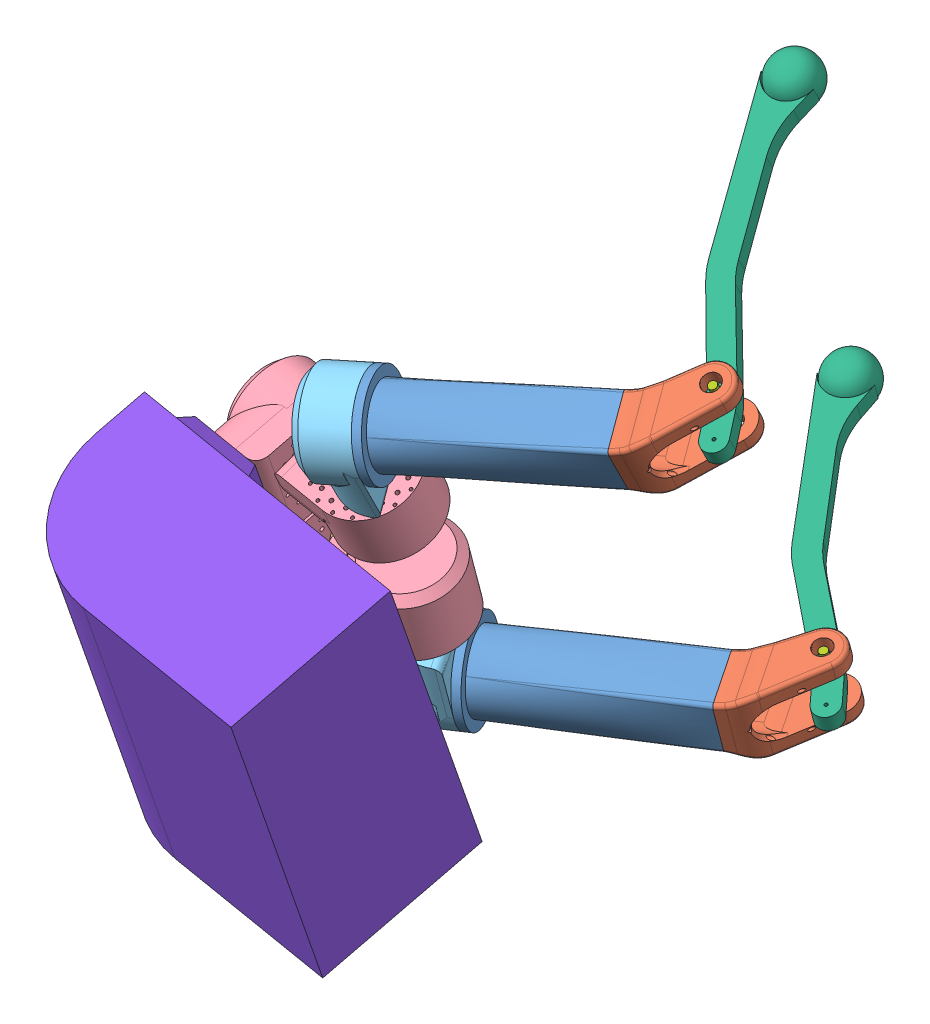
SolidWorks assembly Leg, configuration Default. Lengths in mm.
Overall size (609.04 770.66 944.9).
21 component instances, 8 part files, 41 mates.
Components (placement in the parent):
- Leg_upper-1: Leg_upper [Default] at (371.0813 -601.602 100.7104) x (0.457544 -0.307811 0.83421) z (0.078489 0.94849 0.306929) size (122.65 362.34 115)
  - leg_upper_infront_1-1: leg_upper_infront_1 [Default] at (70.6458 26.5557 199.3325) size (115 250.01 115)
  - leg_upper_infront_2_kfe-1: leg_upper_infront_2_kfe [Default] at (70.6458 26.5557 199.3325) x (0 0 -1) z (1 0 0) size (90 112.35 100.44)
- Output_2-1: Output_2 [Default] at (419.1284 -358.457 248.7598) x (0.995827 -0.088977 0.020306) z (0.04657 0.304055 -0.951516) size (60 8 60)
- Output_2-2: Output_2 [Default] at (343.8426 -295.313 260.2175) x (0.078494 0.948503 0.306888) z (0.105751 0.298179 -0.948634) size (60 8 60)
- Cover_new-1: Cover_new [Default] at (329.9645 -293.8162 259.1409) x (0.071259 0.926481 0.369533) z (0.110755 0.360835 -0.92603) size (115 87.5 130)
- Cover_new-2: Cover_new [Default] at (420.2272 -345.1781 253.0568) x (-0.105755 -0.29822 0.94862) z (0.99129 -0.106915 0.0769) size (115 87.5 130)
- cover-1: cover [Default] at (442.5711 -432.292 208.6587) x (-0.457544 0.307811 -0.83421) z (0.078489 0.94849 0.306929) size (115 63.6 130)
- Leg_Lower_in-1: Leg_Lower_in [Default] at (722.9885 -394.6471 20.617) x (0.638588 -0.284257 0.715125) z (0.765536 0.139872 -0.628005) size (435 60 72.6)
- m10-1: m10 [Default] at (722.9885 -394.6471 20.617) x (0.978231 -0.132605 0.159627) z (0.192105 0.287719 -0.93825) size (10 80 10)
- Leg_upper-2: Leg_upper [Default] at (402.8677 -215.3009 223.9043) x (0.45192 -0.442305 0.774684) z (0.058672 0.88128 0.468939) size (122.65 362.34 115)
  - leg_upper_infront_1-1: leg_upper_infront_1 [Default] at (70.6458 26.5557 199.3325) size (115 250.01 115)
  - leg_upper_infront_2_kfe-1: leg_upper_infront_2_kfe [Default] at (70.6458 26.5557 199.3325) x (0 0 -1) z (1 0 0) size (90 112.35 100.44)
- Output_2-3: Output_2 [Default] at (435.4948 -142.9958 337.3459) x (0.99683 -0.077005 0.019996) z (-0.053733 -0.466279 0.883004) size (60 8 60)
- Output_2-4: Output_2 [Default] at (352.3224 -185.0618 304.192) x (-0.058677 -0.8813 -0.468901) z (-0.117905 -0.460304 0.879897) size (60 8 60)
- Cover_new-3: Cover_new [Default] at (338.4443 -183.565 303.1154) x (0.071259 0.926481 0.369533) z (0.110755 0.360835 -0.92603) size (115 87.5 130)
- Cover_new-4: Cover_new [Default] at (434.6734 -155.3337 330.7808) x (0.117907 0.460343 -0.879876) z (0.99129 -0.106915 0.0769) size (115 87.5 130)
- cover-2: cover [Default] at (470.1271 -66.4594 360.8418) x (0.45192 -0.442305 0.774684) z (-0.058672 -0.88128 -0.468939) size (115 63.6 130)
- Leg_Lower_in-2: Leg_Lower_in [Default] at (752.2584 7.4566 186.6317) x (0.495215 -0.433568 0.752848) z (0.866787 0.188055 -0.461861) size (435 60 72.6)
- m10-2: m10 [Default] at (752.2584 7.4566 186.6317) x (0.982378 -0.134474 0.129807) z (-0.177457 -0.453059 0.87364) size (10 80 10)
- main-2: main [Default] at (417.3182 -308.2316 439.4518) x (0.99129 -0.106915 0.0769) z (0.071259 0.926481 0.369533) size (350 240 400)
Mates (geometry in assembly coordinates):
- Coincident1: coincident anti-aligned: plane of Output_2-2 through (343.8426 -295.313 260.2175) normal (-0.99129 0.106915 -0.0769); plane of Cover_new-1 through (343.8426 -295.313 260.2175) normal (0.99129 -0.106915 0.0769)
- Concentric1: concentric aligned: cylinder of Output_2-2 through (351.7729 -296.1684 260.8327) axis (-0.99129 0.106915 -0.0769) radius 30; cylinder of Cover_new-1 through (343.8426 -295.313 260.2175) axis (-0.99129 0.106915 -0.0769) radius 57.5
- Coincident2: coincident anti-aligned: plane of Output_2-2 through (351.7729 -296.1684 260.8327) normal (0.99129 -0.106915 0.0769); plane of Cover_new-2 through (342.2778 -354.5744 302.0273) normal (-0.99129 0.106915 -0.0769)
- Coincident3: coincident anti-aligned: plane of Output_2-1 through (419.1284 -358.457 248.7598) normal (0.078489 0.94849 0.306929); plane of Cover_new-2 through (419.1284 -358.457 248.7598) normal (-0.078489 -0.94849 -0.306929)
- Concentric2: concentric aligned: cylinder of Output_2-1 through (418.5005 -366.0449 246.3044) axis (0.078489 0.94849 0.306929) radius 30; cylinder of Cover_new-2 through (419.1284 -358.457 248.7598) axis (0.078489 0.94849 0.306929) radius 57.5
- Concentric5: concentric aligned: cylinder of Output_2-2 through (349.3406 -303.0265 282.6513) axis (-0.99129 0.106915 -0.0769) radius 2.1; cylinder of Cover_new-2 through (416.2527 -310.2433 287.842) axis (-0.99129 0.106915 -0.0769) radius 2.25
- Coincident4: coincident anti-aligned: line of Output_2-2 through (352.1202 -280.7044 277.8557) axis (-0.99129 0.106915 -0.0769); line of Cover_new-2 through (362.0331 -281.7735 278.6247) axis (0.99129 -0.106915 0.0769)
- Concentric8: concentric anti-aligned: cylinder of Leg_upper-1/leg_upper_infront_1-1 through (454.6807 -434.343 211.9002) axis (-0.960314 -0.010724 0.278716) radius 57.5; cylinder of cover-1 through (430.6728 -434.6111 218.8681) axis (0.960314 0.010724 -0.278716) radius 57.5
- Coincident5: coincident anti-aligned: plane of Leg_upper-1/leg_upper_infront_1-1 through (445.0775 -434.4502 214.6874) normal (-0.960314 -0.010724 0.278716); plane of cover-1 through (445.0775 -434.4502 214.6874) normal (0.960314 0.010724 -0.278716)
- Coincident6: coincident anti-aligned: plane of Output_2-1 through (418.5005 -366.0449 246.3044) normal (-0.078489 -0.94849 -0.306929); plane of cover-1 through (435.3781 -347.4788 184.6144) normal (0.078489 0.94849 0.306929)
- Concentric9: concentric aligned: line of Output_2-1 through (396.4142 -366.2917 252.7151) axis (0.078489 0.94849 0.306929); cylinder of cover-1 through (390.4805 -437.9976 229.5112) axis (0.078489 0.94849 0.306929) radius 2
- Coincident7: coincident aligned: line of Output_2-1 through (412.7891 -372.4751 267.6359) axis (0.078489 0.94849 0.306929); line of cover-1 through (412.0042 -381.96 264.5666) axis (0.078489 0.94849 0.306929)
- Concentric10: concentric aligned: cylinder of Leg_upper-1/leg_upper_infront_2_kfe-1 through (761.8161 -375.4378 97.94) axis (-0.078489 -0.94849 -0.306929) radius 11; circle of Leg_Lower_in-1
- Coincident9: coincident anti-aligned: plane of cover-1 through (445.0775 -434.4502 214.6874) normal (0.078489 0.94849 0.306929); plane of Leg_Lower_in-1 through (758.2841 -418.1199 84.1282) normal (-0.078489 -0.94849 -0.306929)
- Coincident12: coincident aligned: plane of Leg_upper-1/leg_upper_infront_1-1 through (445.0775 -434.4502 214.6874) normal (0.078489 0.94849 0.306929); plane of cover-1 through (445.0775 -434.4502 214.6874) normal (0.078489 0.94849 0.306929)
- Concentric11: concentric aligned: cylinder of Leg_Lower_in-1 through (759.069 -408.635 87.1975) axis (-0.078489 -0.94849 -0.306929) radius 5; cylinder of m10-1 through (761.4237 -380.1803 96.4054) axis (-0.078489 -0.94849 -0.306929) radius 5
- Coincident13: coincident aligned: plane of Leg_Lower_in-1 through (758.2841 -418.1199 84.1282) normal (-0.078489 -0.94849 -0.306929); plane of m10-1 through (758.2841 -418.1199 84.1282) normal (-0.078489 -0.94849 -0.306929)
- Coincident15: coincident anti-aligned: plane of Output_2-4 through (352.3224 -185.0618 304.192) normal (-0.99129 0.106915 -0.0769); plane of Cover_new-3 through (352.3224 -185.0618 304.192) normal (0.99129 -0.106915 0.0769)
- Concentric13: concentric aligned: cylinder of Output_2-4 through (360.2527 -185.9171 304.8072) axis (-0.99129 0.106915 -0.0769) radius 30; cylinder of Cover_new-3 through (352.3224 -185.0618 304.192) axis (-0.99129 0.106915 -0.0769) radius 57.5
- Coincident16: coincident anti-aligned: plane of Output_2-4 through (360.2527 -185.9171 304.8072) normal (0.99129 -0.106915 0.0769); plane of Cover_new-4 through (369.5845 -121.1126 274.6126) normal (-0.99129 0.106915 -0.0769)
- Coincident17: coincident anti-aligned: plane of Output_2-3 through (435.4948 -142.9958 337.3459) normal (-0.058672 -0.88128 -0.468939); plane of Cover_new-4 through (435.4948 -142.9958 337.3459) normal (0.058672 0.88128 0.468939)
- Concentric14: concentric aligned: cylinder of Output_2-3 through (435.9642 -135.9455 341.0974) axis (-0.058672 -0.88128 -0.468939) radius 30; cylinder of Cover_new-4 through (435.4948 -142.9958 337.3459) axis (-0.058672 -0.88128 -0.468939) radius 57.5
- Coincident18: coincident anti-aligned: plane of Output_2-3 through (435.9642 -135.9455 341.0974) normal (0.058672 0.88128 0.468939); plane of cover-2 through (485.4086 -159.4246 379.0356) normal (-0.058672 -0.88128 -0.468939)
- Coincident19: coincident aligned: plane of cover-2 through (472.1645 -68.899 365.1717) normal (-0.058672 -0.88128 -0.468939); plane of Leg_Lower_in-2 through (780.6779 -18.6376 232.1151) normal (-0.058672 -0.88128 -0.468939)
- Concentric15: concentric anti-aligned: cylinder of Leg_Lower_in-2 through (781.2646 -9.8248 236.8045) axis (-0.058672 -0.88128 -0.468939) radius 5; cylinder of m10-2 through (778.331 -53.8888 213.3575) axis (0.058672 0.88128 0.468939) radius 5
- Coincident20: coincident anti-aligned: plane of Leg_Lower_in-2 through (780.6779 -18.6376 232.1151) normal (-0.058672 -0.88128 -0.468939); plane of m10-2 through (780.6779 -18.6376 232.1151) normal (0.058672 0.88128 0.468939)
- Concentric16: concentric anti-aligned: cylinder of Leg_upper-2/leg_upper_infront_2_kfe-1 through (783.3181 21.0199 253.2174) axis (-0.058672 -0.88128 -0.468939) radius 11; cylinder of m10-2 through (778.331 -53.8888 213.3575) axis (0.058672 0.88128 0.468939) radius 5
- Coincident21: coincident anti-aligned: plane of Leg_upper-2/leg_upper_infront_1-1 through (472.1645 -68.899 365.1717) normal (-0.950765 -0.093865 0.295358); plane of cover-2 through (472.1645 -68.899 365.1717) normal (0.950765 0.093865 -0.295358)
- Concentric17: concentric anti-aligned: cylinder of Leg_upper-2/leg_upper_infront_1-1 through (481.6722 -67.9604 362.2181) axis (-0.950765 -0.093865 0.295358) radius 57.5; cylinder of cover-2 through (457.9031 -70.307 369.602) axis (0.950765 0.093865 -0.295358) radius 57.5
- Coincident22: coincident anti-aligned: plane of Output_2-3 through (435.9642 -135.9455 341.0974) normal (0.058672 0.88128 0.468939); plane of cover-2 through (485.4086 -159.4246 379.0356) normal (-0.058672 -0.88128 -0.468939)
- Concentric19: concentric aligned: cylinder of Output_2-4 through (362.9645 -175.3301 284.5695) axis (-0.99129 0.106915 -0.0769) radius 2.1; line of Cover_new-4 through (372.8774 -176.3993 285.3385) axis (-0.99129 0.106915 -0.0769)
- Concentric22: concentric anti-aligned: cylinder of Output_2-4 through (360.4399 -198.1779 285.3475) axis (-0.99129 0.106915 -0.0769) radius 2.1; cylinder of Cover_new-4 through (370.3528 -199.247 286.1165) axis (0.99129 -0.106915 0.0769) radius 4.5
- Concentric23: concentric aligned: cylinder of Output_2-3 through (452.9603 -144.0921 354.2809) axis (-0.058672 -0.88128 -0.468939) radius 2.1; cylinder of cover-2 through (457.3959 -77.4674 389.7327) axis (-0.058672 -0.88128 -0.468939) radius 2
- Concentric24: concentric aligned: cylinder of Output_2-3 through (414.0975 -138.1046 347.8908) axis (-0.058672 -0.88128 -0.468939) radius 2.1; cylinder of cover-2 through (418.5331 -71.4798 383.3426) axis (-0.058672 -0.88128 -0.468939) radius 2
- Parallel1: parallel aligned: plane of Cover_new-1 through (257.6004 -286.0114 253.5272) normal (-0.99129 0.106915 -0.0769); plane of Cover_new-3 through (266.0802 -175.7601 297.5016) normal (-0.99129 0.106915 -0.0769)
- Coincident23: coincident anti-aligned: plane of Cover_new-3 through (334.5119 -156.4528 391.5007) normal (-0.110755 -0.360835 0.92603); plane of main-2 through (283.9529 134.8553 498.9642) normal (0.110755 0.360835 -0.92603)
- Coincident24: coincident aligned: plane of Cover_new-3 through (266.0802 -175.7601 297.5016) normal (-0.99129 0.106915 -0.0769); plane of main-2 through (218.892 -452.0449 521.6634) normal (-0.99129 0.106915 -0.0769)
- Coincident25: coincident: plane of Cover_new-3 through (356.4197 -131.7891 325.4401) normal (0.071259 0.926481 0.369533); line of main-2 through (346.4074 -157.7358 392.4235) axis (-0.99129 0.106915 -0.0769)
- Coincident26: coincident aligned: plane of Cover_new-1 through (257.6004 -286.0114 253.5272) normal (-0.99129 0.106915 -0.0769); plane of main-2 through (218.892 -452.0449 521.6634) normal (-0.99129 0.106915 -0.0769)
- Coincident27: coincident anti-aligned: plane of Cover_new-1 through (326.0321 -266.7041 347.5262) normal (-0.110755 -0.360835 0.92603); plane of main-2 through (283.9529 134.8553 498.9642) normal (0.110755 0.360835 -0.92603)
- Coincident28: coincident: plane of Cover_new-1 through (339.7452 -348.5857 238.9693) normal (-0.071259 -0.926481 -0.369533); line of main-2 through (329.7329 -374.5324 305.9527) axis (-0.99129 0.106915 -0.0769)
